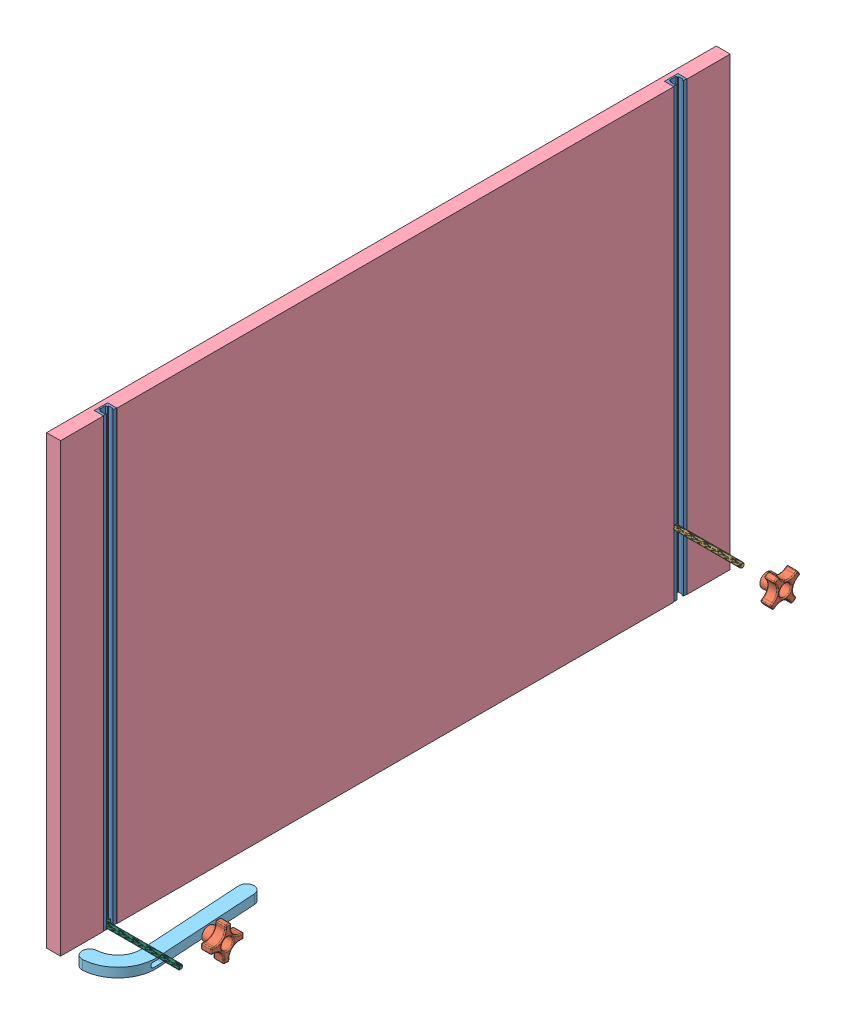
SolidWorks assembly CNCHolderAssembly, configuration Default. Lengths in mm.
Overall size (185.8 627.06 914.4).
8 component instances, 6 part files, 5 mates.
Components (placement in the parent):
- 1850A14_24  Long T-Track Fixturing Track-1: 1850A14_24  Long T-Track Fixturing Track [1850A14] at (-456.3718 -340.4631 495.8829) x (0 -1 0) z (1 0 0) size (609.6 18.29 12.19)
- 1850A14_24  Long T-Track Fixturing Track-2: 1850A14_24  Long T-Track Fixturing Track [1850A14] at (-456.3718 -340.4631 -282.7541) x (0 -1 0) z (1 0 0) size (609.6 18.29 12.19)
- 7921K616_Nylon Four Arm Knob-1: 7921K616_Nylon Four Arm Knob [7921K616] at (-313.283 -558.2426 -276.5863) x (0 -0.836045 -0.548661) z (1 0 0) size (44.45 44.45 25.7)
- 92800A363_18-8 Stainless Steel Hex Head Screw-1: 92800A363_18-8 Stainless Steel Hex Head Screw [92800A363] at (-448.1485 -558.2426 -276.5863) x (0 0.989106 -0.147204) z (-1 0 0) size (11.11 13.98 100.2)
- 1125T525_Cdx Grade Plywood Sheet-1: 1125T525_Cdx Grade Plywood Sheet [1125T525] at (-462.7218 -340.4631 106.5644) x (0 1 0) z (0 0 1) size (609.6 19.05 914.4)
- 7921K616_Nylon Four Arm Knob-2: 7921K616_Nylon Four Arm Knob [7921K616] at (-295.9756 -578.0268 502.509) x (0 -0.060023 -0.998197) z (1 0 0) size (44.45 44.45 25.7)
- Part2^CNCHolderAssembly-1: Part2^CNCHolderAssembly [Default] at (41.5153 385.7997 2.1261) x (0.996488 0.057273 -0.061084) z (0.061552 -0.006436 0.998083) size (62.3 17.39 202.36) (virtual)
- 92865A558_Medium-Strength Grade 5 Steel Hex Head Screw-1: 92865A558_Medium-Strength Grade 5 Steel Hex Head Screw [92865A558] at (-398.1828 -642.1462 497.9088) x (0 0 1) z (-1 0 0) size (11.11 12.83 106.8)
Mates (geometry in assembly coordinates):
- Coincident36: coincident anti-aligned: plane of 1850A14_24  Long T-Track Fixturing Track-2 through (-452.1173 -645.2631 -288.7231) normal (1 0 0); plane of 92800A363_18-8 Stainless Steel Hex Head Screw-1 through (-452.1173 -558.2426 -276.5863) normal (-1 0 0)
- Screw2: screw = 1 aligned: cone of 7921K616_Nylon Four Arm Knob-1 through (-319.633 -558.2426 -276.5863) axis (1 0 0); cone of 92800A363_18-8 Stainless Steel Hex Head Screw-1 through (-352.8985 -558.2426 -276.5863) axis (1 0 0)
- Coincident39: coincident anti-aligned: plane of 1850A14_24  Long T-Track Fixturing Track-1 through (-456.3718 -645.2631 505.0269) normal (-1 0 0); plane of 1125T525_Cdx Grade Plywood Sheet-1 through (-456.3718 -340.4631 106.5644) normal (1 0 0)
- Coincident40: coincident: point of 1850A14_24  Long T-Track Fixturing Track-1; point of 1125T525_Cdx Grade Plywood Sheet-1
- Coincident41: coincident: point of 1850A14_24  Long T-Track Fixturing Track-2; point of 1125T525_Cdx Grade Plywood Sheet-1
